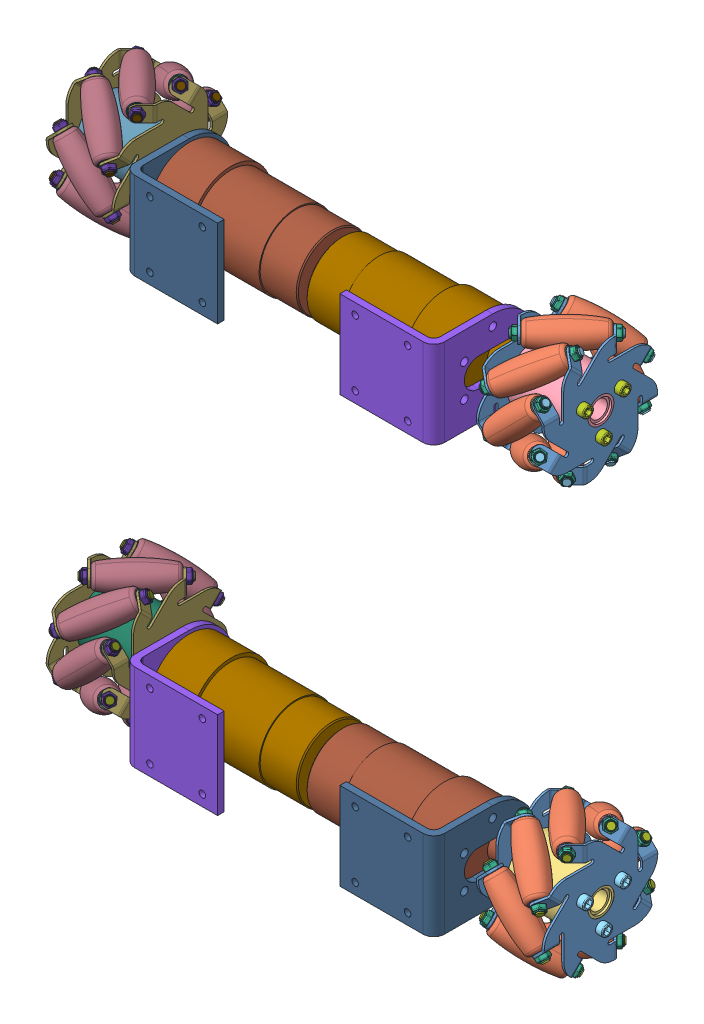
SolidWorks assembly car, configuration 默认. Lengths in mm. (continued)
Components (placement in the parent): (continued)
- Tank(2)^car-1: Tank(2)^car [默认] at origin size (280 382.88 170.83) (virtual) (continued)
  - Mecanum_Wheel_60mm_Left_ASM_AP214 v1 (1)^Tank(2)_car-1: Mecanum_Wheel_60mm_Left_ASM_AP214 v1 (1)^Tank(2)_car [默认] at (89.5247 -221.4281 -134.5883) x (1 0 0) z (0 -0.707107 -0.707107) size (37 63.14 63.14) (virtual) (continued)
    - roller_Varsayilan (1)^Mecanum_Wheel_60mm_Left_ASM_AP214 v1 (1)_Tank(2)_car-2: roller_Varsayilan (1)^Mecanum_Wheel_60mm_Left_ASM_AP214 v1 (1)_Tank(2)_car [默认] at (-11.1205 22.2762 30.2518) x (0.707107 0 0.707107) z (-0.228848 -0.94618 0.228848) size (29.8 12.94 12.94) (virtual)
    - roller_Varsayilan (1)^Mecanum_Wheel_60mm_Left_ASM_AP214 v1 (1)_Tank(2)_car-3: roller_Varsayilan (1)^Mecanum_Wheel_60mm_Left_ASM_AP214 v1 (1)_Tank(2)_car [默认] at (-11.1205 15.7922 13.8838) x (0.707107 0.5 0.5) z (-0.228848 -0.50723 0.830871) size (29.8 12.94 12.94) (virtual)
    - roller_Varsayilan (1)^Mecanum_Wheel_60mm_Left_ASM_AP214 v1 (1)_Tank(2)_car-4: roller_Varsayilan (1)^Mecanum_Wheel_60mm_Left_ASM_AP214 v1 (1)_Tank(2)_car [默认] at (-11.1205 -0.3667 6.8948) x (0.707107 0.707107 0) z (-0.228848 0.228848 0.94618) size (29.8 12.94 12.94) (virtual)
    - roller_Varsayilan (1)^Mecanum_Wheel_60mm_Left_ASM_AP214 v1 (1)_Tank(2)_car-5: roller_Varsayilan (1)^Mecanum_Wheel_60mm_Left_ASM_AP214 v1 (1)_Tank(2)_car [默认] at (-11.1205 -16.7348 13.3789) x (0.707107 0.5 -0.5) z (-0.228848 0.830871 0.50723) size (29.8 12.94 12.94) (virtual)
    - roller_Varsayilan (1)^Mecanum_Wheel_60mm_Left_ASM_AP214 v1 (1)_Tank(2)_car-6: roller_Varsayilan (1)^Mecanum_Wheel_60mm_Left_ASM_AP214 v1 (1)_Tank(2)_car [默认] at (-11.1205 -23.7238 29.5377) x (0.707107 0 -0.707107) z (-0.228848 0.94618 -0.228848) size (29.8 12.94 12.94) (virtual)
    - roller_Varsayilan (1)^Mecanum_Wheel_60mm_Left_ASM_AP214 v1 (1)_Tank(2)_car-7: roller_Varsayilan (1)^Mecanum_Wheel_60mm_Left_ASM_AP214 v1 (1)_Tank(2)_car [默认] at (-11.1205 -17.2397 45.9058) x (0.707107 -0.5 -0.5) z (-0.228848 0.50723 -0.830871) size (29.8 12.94 12.94) (virtual)
    - roller_Varsayilan (1)^Mecanum_Wheel_60mm_Left_ASM_AP214 v1 (1)_Tank(2)_car-8: roller_Varsayilan (1)^Mecanum_Wheel_60mm_Left_ASM_AP214 v1 (1)_Tank(2)_car [默认] at (-11.1205 -1.0808 52.8948) x (0.707107 -0.707107 0) z (-0.228848 -0.228848 -0.94618) size (29.8 12.94 12.94) (virtual)
    - 3x35_screw_Varsayilan (1)^Mecanum_Wheel_60mm_Left_ASM_AP214 v1 (1)_Tank(2)_car-2: 3x35_screw_Varsayilan (1)^Mecanum_Wheel_60mm_Left_ASM_AP214 v1 (1)_Tank(2)_car [默认] at (-29.9304 1.8644 20.2355) x (0 -0.866025 0.5) z (1 0 0) size (5 5 37) (virtual)
    - 3x35_screw_Varsayilan (1)^Mecanum_Wheel_60mm_Left_ASM_AP214 v1 (1)_Tank(2)_car-3: 3x35_screw_Varsayilan (1)^Mecanum_Wheel_60mm_Left_ASM_AP214 v1 (1)_Tank(2)_car [默认] at (-29.9304 -10.383 32.483) x (0 0.866025 0.5) z (1 0 0) size (5 5 37) (virtual)
    - 3mm_bolt_Varsayilan (1)^Mecanum_Wheel_60mm_Left_ASM_AP214 v1 (1)_Tank(2)_car-2: 3mm_bolt_Varsayilan (1)^Mecanum_Wheel_60mm_Left_ASM_AP214 v1 (1)_Tank(2)_car [默认] at (-27.0247 -10.383 32.483) x (0 -0.940173 -0.340697) z (-1 0 0) size (5.6 5.2 2.5) (virtual)
    - 3mm_bolt_Varsayilan (1)^Mecanum_Wheel_60mm_Left_ASM_AP214 v1 (1)_Tank(2)_car-3: 3mm_bolt_Varsayilan (1)^Mecanum_Wheel_60mm_Left_ASM_AP214 v1 (1)_Tank(2)_car [默认] at (-27.0247 6.3473 36.9659) x (0 0.175035 0.984562) z (-1 0 0) size (5.6 5.2 2.5) (virtual)
    - 3mm_bolt_Varsayilan (1)^Mecanum_Wheel_60mm_Left_ASM_AP214 v1 (1)_Tank(2)_car-4: 3mm_bolt_Varsayilan (1)^Mecanum_Wheel_60mm_Left_ASM_AP214 v1 (1)_Tank(2)_car [默认] at (-22.8133 7.5242 5.6158) x (-0.060636 0.747379 -0.661626) z (-0.707107 -0.5 -0.5) size (5.6 5.2 2.5) (virtual)
    - 3mm_bolt_Varsayilan (1)^Mecanum_Wheel_60mm_Left_ASM_AP214 v1 (1)_Tank(2)_car-5: 3mm_bolt_Varsayilan (1)^Mecanum_Wheel_60mm_Left_ASM_AP214 v1 (1)_Tank(2)_car [默认] at (-0.1419 23.5552 21.6469) x (0.267213 0.465725 -0.843622) z (0.707107 0.5 0.5) size (5.6 5.2 2.5) (virtual)
    - 3mm_bolt_Varsayilan (1)^Mecanum_Wheel_60mm_Left_ASM_AP214 v1 (1)_Tank(2)_car-6: 3mm_bolt_Varsayilan (1)^Mecanum_Wheel_60mm_Left_ASM_AP214 v1 (1)_Tank(2)_car [默认] at (-22.8133 22.2762 18.5591) x (-0.060636 0.996316 0.060636) z (-0.707107 0 -0.707107) size (5.6 5.2 2.5) (virtual)
    - 3mm_bolt_Varsayilan (1)^Mecanum_Wheel_60mm_Left_ASM_AP214 v1 (1)_Tank(2)_car-7: 3mm_bolt_Varsayilan (1)^Mecanum_Wheel_60mm_Left_ASM_AP214 v1 (1)_Tank(2)_car [默认] at (-22.8133 23.5552 38.1427) x (-0.060636 0.661626 0.747379) z (-0.707107 0.5 -0.5) size (5.6 5.2 2.5) (virtual)
    - 3mm_bolt_Varsayilan (1)^Mecanum_Wheel_60mm_Left_ASM_AP214 v1 (1)_Tank(2)_car-8: 3mm_bolt_Varsayilan (1)^Mecanum_Wheel_60mm_Left_ASM_AP214 v1 (1)_Tank(2)_car [默认] at (-22.8133 10.6119 52.8948) x (-0.060636 -0.060636 0.996316) z (-0.707107 0.707107 0) size (5.6 5.2 2.5) (virtual)
    - 3mm_bolt_Varsayilan (1)^Mecanum_Wheel_60mm_Left_ASM_AP214 v1 (1)_Tank(2)_car-9: 3mm_bolt_Varsayilan (1)^Mecanum_Wheel_60mm_Left_ASM_AP214 v1 (1)_Tank(2)_car [默认] at (-22.8133 -8.9717 54.1738) x (-0.060636 -0.747379 0.661626) z (-0.707107 0.5 0.5) size (5.6 5.2 2.5) (virtual)
    - 3mm_bolt_Varsayilan (1)^Mecanum_Wheel_60mm_Left_ASM_AP214 v1 (1)_Tank(2)_car-10: 3mm_bolt_Varsayilan (1)^Mecanum_Wheel_60mm_Left_ASM_AP214 v1 (1)_Tank(2)_car [默认] at (-22.8133 -23.7238 41.2305) x (-0.060636 -0.996316 -0.060636) z (-0.707107 0 0.707107) size (5.6 5.2 2.5) (virtual)
    - 3mm_bolt_Varsayilan (1)^Mecanum_Wheel_60mm_Left_ASM_AP214 v1 (1)_Tank(2)_car-11: 3mm_bolt_Varsayilan (1)^Mecanum_Wheel_60mm_Left_ASM_AP214 v1 (1)_Tank(2)_car [默认] at (-22.8133 -25.0028 21.6469) x (-0.060636 -0.661626 -0.747379) z (-0.707107 -0.5 0.5) size (5.6 5.2 2.5) (virtual)
    - 3mm_bolt_Varsayilan (1)^Mecanum_Wheel_60mm_Left_ASM_AP214 v1 (1)_Tank(2)_car-12: 3mm_bolt_Varsayilan (1)^Mecanum_Wheel_60mm_Left_ASM_AP214 v1 (1)_Tank(2)_car [默认] at (-22.8133 -12.0594 6.8948) x (-0.060636 0.060636 -0.996316) z (-0.707107 -0.707107 0) size (5.6 5.2 2.5) (virtual)
    - 3mm_bolt_Varsayilan (1)^Mecanum_Wheel_60mm_Left_ASM_AP214 v1 (1)_Tank(2)_car-13: 3mm_bolt_Varsayilan (1)^Mecanum_Wheel_60mm_Left_ASM_AP214 v1 (1)_Tank(2)_car [默认] at (-0.1419 22.2762 41.2305) x (0.267213 0.925848 -0.267213) z (0.707107 0 0.707107) size (5.6 5.2 2.5) (virtual)
    - 3mm_bolt_Varsayilan (1)^Mecanum_Wheel_60mm_Left_ASM_AP214 v1 (1)_Tank(2)_car-14: 3mm_bolt_Varsayilan (1)^Mecanum_Wheel_60mm_Left_ASM_AP214 v1 (1)_Tank(2)_car [默认] at (-0.1419 7.5242 54.1738) x (0.267213 0.843622 0.465725) z (0.707107 -0.5 0.5) size (5.6 5.2 2.5) (virtual)
    - 3mm_bolt_Varsayilan (1)^Mecanum_Wheel_60mm_Left_ASM_AP214 v1 (1)_Tank(2)_car-15: 3mm_bolt_Varsayilan (1)^Mecanum_Wheel_60mm_Left_ASM_AP214 v1 (1)_Tank(2)_car [默认] at (-0.1419 -12.0594 52.8948) x (0.267213 0.267213 0.925848) z (0.707107 -0.707107 0) size (5.6 5.2 2.5) (virtual)
    - 3mm_bolt_Varsayilan (1)^Mecanum_Wheel_60mm_Left_ASM_AP214 v1 (1)_Tank(2)_car-16: 3mm_bolt_Varsayilan (1)^Mecanum_Wheel_60mm_Left_ASM_AP214 v1 (1)_Tank(2)_car [默认] at (-0.1419 -25.0028 38.1427) x (0.267213 -0.465725 0.843622) z (0.707107 -0.5 -0.5) size (5.6 5.2 2.5) (virtual)
    - 3mm_bolt_Varsayilan (1)^Mecanum_Wheel_60mm_Left_ASM_AP214 v1 (1)_Tank(2)_car-17: 3mm_bolt_Varsayilan (1)^Mecanum_Wheel_60mm_Left_ASM_AP214 v1 (1)_Tank(2)_car [默认] at (-0.1419 -23.7238 18.5591) x (0.267213 -0.925848 0.267213) z (0.707107 0 -0.707107) size (5.6 5.2 2.5) (virtual)
    - 3mm_bolt_Varsayilan (1)^Mecanum_Wheel_60mm_Left_ASM_AP214 v1 (1)_Tank(2)_car-18: 3mm_bolt_Varsayilan (1)^Mecanum_Wheel_60mm_Left_ASM_AP214 v1 (1)_Tank(2)_car [默认] at (-0.1419 -8.9717 5.6158) x (0.267213 -0.843622 -0.465725) z (0.707107 0.5 -0.5) size (5.6 5.2 2.5) (virtual)
    - 3mm_bolt_Varsayilan (1)^Mecanum_Wheel_60mm_Left_ASM_AP214 v1 (1)_Tank(2)_car-19: 3mm_bolt_Varsayilan (1)^Mecanum_Wheel_60mm_Left_ASM_AP214 v1 (1)_Tank(2)_car [默认] at (-0.1419 10.6119 6.8948) x (0.267213 -0.267213 -0.925848) z (0.707107 0.707107 0) size (5.6 5.2 2.5) (virtual)
    - two_sided_screw_Varsayilan (1)^Mecanum_Wheel_60mm_Left_ASM_AP214 v1 (1)_Tank(2)_car-2: two_sided_screw_Varsayilan (1)^Mecanum_Wheel_60mm_Left_ASM_AP214 v1 (1)_Tank(2)_car [默认] at (-24.8906 22.2762 16.4817) x (-0.576606 0.578837 0.576606) z (0.707107 0 0.707107) size (3 3 38) (virtual)
    - two_sided_screw_Varsayilan (1)^Mecanum_Wheel_60mm_Left_ASM_AP214 v1 (1)_Tank(2)_car-3: two_sided_screw_Varsayilan (1)^Mecanum_Wheel_60mm_Left_ASM_AP214 v1 (1)_Tank(2)_car [默认] at (-24.8906 25.0242 36.6738) x (-0.576606 0.001578 0.817021) z (0.707107 -0.5 0.5) size (3 3 38) (virtual)
    - two_sided_screw_Varsayilan (1)^Mecanum_Wheel_60mm_Left_ASM_AP214 v1 (1)_Tank(2)_car-4: two_sided_screw_Varsayilan (1)^Mecanum_Wheel_60mm_Left_ASM_AP214 v1 (1)_Tank(2)_car [默认] at (-24.8906 12.6893 52.8948) x (-0.576606 -0.576606 0.578837) z (0.707107 -0.707107 0) size (3 3 38) (virtual)
    - two_sided_screw_Varsayilan (1)^Mecanum_Wheel_60mm_Left_ASM_AP214 v1 (1)_Tank(2)_car-5: two_sided_screw_Varsayilan (1)^Mecanum_Wheel_60mm_Left_ASM_AP214 v1 (1)_Tank(2)_car [默认] at (-24.8906 -7.5028 55.6427) x (-0.576606 -0.817021 0.001578) z (0.707107 -0.5 -0.5) size (3 3 38) (virtual)
    - two_sided_screw_Varsayilan (1)^Mecanum_Wheel_60mm_Left_ASM_AP214 v1 (1)_Tank(2)_car-6: two_sided_screw_Varsayilan (1)^Mecanum_Wheel_60mm_Left_ASM_AP214 v1 (1)_Tank(2)_car [默认] at (-24.8906 -23.7238 43.3078) x (-0.576606 -0.578837 -0.576606) z (0.707107 0 -0.707107) size (3 3 38) (virtual)
    - two_sided_screw_Varsayilan (1)^Mecanum_Wheel_60mm_Left_ASM_AP214 v1 (1)_Tank(2)_car-7: two_sided_screw_Varsayilan (1)^Mecanum_Wheel_60mm_Left_ASM_AP214 v1 (1)_Tank(2)_car [默认] at (-24.8906 -26.4717 23.1158) x (-0.576606 -0.001578 -0.817021) z (0.707107 0.5 -0.5) size (3 3 38) (virtual)
    - two_sided_screw_Varsayilan (1)^Mecanum_Wheel_60mm_Left_ASM_AP214 v1 (1)_Tank(2)_car-8: two_sided_screw_Varsayilan (1)^Mecanum_Wheel_60mm_Left_ASM_AP214 v1 (1)_Tank(2)_car [默认] at (-24.8906 -14.1368 6.8948) x (-0.576606 0.576606 -0.578837) z (0.707107 0.707107 0) size (3 3 38) (virtual)
  - DC LF (1)^Tank(2)_car-1: DC LF (1)^Tank(2)_car [默认] at (-41 -242.0551 -178.2389) x (-1 0 0) z (0 0 1) size (95 40 47) (virtual)
    - Component10(Mirror)^DC LF (1)_Tank(2)_car-1: Component10(Mirror)^DC LF (1)_Tank(2)_car [默认] at origin size (43 40 47) (virtual)
    - DC LF (1)-2^DC LF (1)_Tank(2)_car-1: DC LF (1)-2^DC LF (1)_Tank(2)_car [默认] at origin size (95 37 37) (virtual)
  - DC RF (1)^Tank(2)_car-1: DC RF (1)^Tank(2)_car [默认] at (0 -242.0551 -178.2389) x (1 0 0) z (0 0 -1) size (95 40 47) (virtual)
    - Component10^DC RF (1)_Tank(2)_car-1: Component10^DC RF (1)_Tank(2)_car [默认] at origin size (43 40 47) (virtual)
    - DC RF (1)-3^DC RF (1)_Tank(2)_car-1: DC RF (1)-3^DC RF (1)_Tank(2)_car [默认] at origin size (95 37 37) (virtual)
  - Mecanum_Wheel_60mm_Right_ASM_AP214 v1 (1)^Tank(2)_car-1: Mecanum_Wheel_60mm_Right_ASM_AP214 v1 (1)^Tank(2)_car [默认] at (-134.5 -218.5276 -89.1195) x (1 0 0) z (0 0 -1) size (83 63.25 63.25) (virtual)
    - plate_2_Varsayilan^Mecanum_Wheel_60mm_Right_ASM_AP214 v1 (1)_Tank(2)_car-1: plate_2_Varsayilan^Mecanum_Wheel_60mm_Right_ASM_AP214 v1 (1)_Tank(2)_car [默认] at (56.8037 4.8798 97.2247) x (0.707107 0.707107 0) z (0 0 1) size (41.63 41.63 53.77) (virtual)
    - roller_Varsayilan^Mecanum_Wheel_60mm_Right_ASM_AP214 v1 (1)_Tank(2)_car-1: roller_Varsayilan^Mecanum_Wheel_60mm_Right_ASM_AP214 v1 (1)_Tank(2)_car [默认] at (15.1622 40.0059 51.0708) x (-0.707107 0.5 0.5) z (-0.704237 -0.434326 -0.561615) size (29.8 12.94 12.94) (virtual)
    - liner_Varsayilan^Mecanum_Wheel_60mm_Right_ASM_AP214 v1 (1)_Tank(2)_car-1: liner_Varsayilan^Mecanum_Wheel_60mm_Right_ASM_AP214 v1 (1)_Tank(2)_car [默认] at (4.8906 47.2689 58.3339) x (-0.663539 -0.224823 -0.713562) z (-0.24437 -0.836334 0.490743) size (7 1 7) (virtual)
    - inner_cylinder_Varsayilan^Mecanum_Wheel_60mm_Right_ASM_AP214 v1 (1)_Tank(2)_car-1: inner_cylinder_Varsayilan^Mecanum_Wheel_60mm_Right_ASM_AP214 v1 (1)_Tank(2)_car [默认] at (30 23.5276 67.1195) x (0 0 1) z (-1 0 0) size (26 26 31) (virtual)
    - two_sided_screw_Varsayilan^Mecanum_Wheel_60mm_Right_ASM_AP214 v1 (1)_Tank(2)_car-1: two_sided_screw_Varsayilan^Mecanum_Wheel_60mm_Right_ASM_AP214 v1 (1)_Tank(2)_car [默认] at (28.9323 30.2689 41.3339) x (-0.195015 0.541787 -0.817579) z (-0.707107 0.5 0.5) size (3 3 38) (virtual)
    - 3mm_bolt_Varsayilan^Mecanum_Wheel_60mm_Right_ASM_AP214 v1 (1)_Tank(2)_car-1: 3mm_bolt_Varsayilan^Mecanum_Wheel_60mm_Right_ASM_AP214 v1 (1)_Tank(2)_car [默认] at (4.155 47.7891 58.854) x (0.638071 0.755922 0.146447) z (-0.707107 0.5 0.5) size (5.6 5.2 2.5) (virtual)
    - 3x35_screw_Varsayilan^Mecanum_Wheel_60mm_Right_ASM_AP214 v1 (1)_Tank(2)_car-1: 3x35_screw_Varsayilan^Mecanum_Wheel_60mm_Right_ASM_AP214 v1 (1)_Tank(2)_car [默认] at (-3 18.5276 58.4592) x (0 0.745603 -0.666391) z (1 0 0) size (5 5 37) (virtual)
    - plate_2_Varsayilan^Mecanum_Wheel_60mm_Right_ASM_AP214 v1 (1)_Tank(2)_car-2: plate_2_Varsayilan^Mecanum_Wheel_60mm_Right_ASM_AP214 v1 (1)_Tank(2)_car [默认] at (-25.8037 4.8798 37.0142) x (-0.707107 0.707107 0) z (0 0 -1) size (41.63 41.63 53.77) (virtual)
    - liner_Varsayilan^Mecanum_Wheel_60mm_Right_ASM_AP214 v1 (1)_Tank(2)_car-2: liner_Varsayilan^Mecanum_Wheel_60mm_Right_ASM_AP214 v1 (1)_Tank(2)_car [默认] at (26.1038 32.2689 43.3339) x (0.54662 -0.062042 0.835079) z (-0.448561 -0.8638 0.22944) size (7 1 7) (virtual)
    - 3mm_bolt_Varsayilan^Mecanum_Wheel_60mm_Right_ASM_AP214 v1 (1)_Tank(2)_car-2: 3mm_bolt_Varsayilan^Mecanum_Wheel_60mm_Right_ASM_AP214 v1 (1)_Tank(2)_car [默认] at (26.8109 31.7689 42.8339) x (0.358192 -0.356391 0.862951) z (0.707107 -0.5 -0.5) size (5.6 5.2 2.5) (virtual)
    - 3mm_bolt_Varsayilan^Mecanum_Wheel_60mm_Right_ASM_AP214 v1 (1)_Tank(2)_car-3: 3mm_bolt_Varsayilan^Mecanum_Wheel_60mm_Right_ASM_AP214 v1 (1)_Tank(2)_car [默认] at (0 18.5276 75.7797) x (0 -0.80734 0.590087) z (-1 0 0) size (5.6 5.2 2.5) (virtual)
    - 3x35_screw_Varsayilan^Mecanum_Wheel_60mm_Right_ASM_AP214 v1 (1)_Tank(2)_car-2: 3x35_screw_Varsayilan^Mecanum_Wheel_60mm_Right_ASM_AP214 v1 (1)_Tank(2)_car [默认] at (-3 18.5276 75.7797) x (0 -0.949913 -0.312516) z (1 0 0) size (5 5 37) (virtual)
    - 3x35_screw_Varsayilan^Mecanum_Wheel_60mm_Right_ASM_AP214 v1 (1)_Tank(2)_car-3: 3x35_screw_Varsayilan^Mecanum_Wheel_60mm_Right_ASM_AP214 v1 (1)_Tank(2)_car [默认] at (-3 33.5276 67.1195) x (0 0.20431 0.978906) z (1 0 0) size (5 5 37) (virtual)
    - 3mm_bolt_Varsayilan^Mecanum_Wheel_60mm_Right_ASM_AP214 v1 (1)_Tank(2)_car-4: 3mm_bolt_Varsayilan^Mecanum_Wheel_60mm_Right_ASM_AP214 v1 (1)_Tank(2)_car [默认] at (0 33.5276 67.1195) x (0 0.9147 0.404133) z (-1 0 0) size (5.6 5.2 2.5) (virtual)
    - 3mm_bolt_Varsayilan^Mecanum_Wheel_60mm_Right_ASM_AP214 v1 (1)_Tank(2)_car-5: 3mm_bolt_Varsayilan^Mecanum_Wheel_60mm_Right_ASM_AP214 v1 (1)_Tank(2)_car [默认] at (0 18.5276 58.4592) x (0 -0.107361 -0.99422) z (-1 0 0) size (5.6 5.2 2.5) (virtual)
    - two_sided_screw_Varsayilan^Mecanum_Wheel_60mm_Right_ASM_AP214 v1 (1)_Tank(2)_car-2: two_sided_screw_Varsayilan^Mecanum_Wheel_60mm_Right_ASM_AP214 v1 (1)_Tank(2)_car [默认] at (28.9323 10.0613 44.1195) x (-0.195015 -0.195015 -0.961217) z (-0.707107 0.707107 0) size (3 3 38) (virtual)
    - two_sided_screw_Varsayilan^Mecanum_Wheel_60mm_Right_ASM_AP214 v1 (1)_Tank(2)_car-3: two_sided_screw_Varsayilan^Mecanum_Wheel_60mm_Right_ASM_AP214 v1 (1)_Tank(2)_car [默认] at (28.9323 -2.258 60.3781) x (-0.195015 -0.817579 -0.541787) z (-0.707107 0.5 -0.5) size (3 3 38) (virtual)
    - two_sided_screw_Varsayilan^Mecanum_Wheel_60mm_Right_ASM_AP214 v1 (1)_Tank(2)_car-4: two_sided_screw_Varsayilan^Mecanum_Wheel_60mm_Right_ASM_AP214 v1 (1)_Tank(2)_car [默认] at (28.9323 0.5276 80.5857) x (-0.195015 -0.961217 0.195015) z (-0.707107 0 -0.707107) size (3 3 38) (virtual)
    - two_sided_screw_Varsayilan^Mecanum_Wheel_60mm_Right_ASM_AP214 v1 (1)_Tank(2)_car-5: two_sided_screw_Varsayilan^Mecanum_Wheel_60mm_Right_ASM_AP214 v1 (1)_Tank(2)_car [默认] at (28.9323 16.7862 92.905) x (-0.195015 -0.541787 0.817579) z (-0.707107 -0.5 -0.5) size (3 3 38) (virtual)
    - two_sided_screw_Varsayilan^Mecanum_Wheel_60mm_Right_ASM_AP214 v1 (1)_Tank(2)_car-6: two_sided_screw_Varsayilan^Mecanum_Wheel_60mm_Right_ASM_AP214 v1 (1)_Tank(2)_car [默认] at (28.9323 36.9938 90.1195) x (-0.195015 0.195015 0.961217) z (-0.707107 -0.707107 0) size (3 3 38) (virtual)
    - two_sided_screw_Varsayilan^Mecanum_Wheel_60mm_Right_ASM_AP214 v1 (1)_Tank(2)_car-7: two_sided_screw_Varsayilan^Mecanum_Wheel_60mm_Right_ASM_AP214 v1 (1)_Tank(2)_car [默认] at (28.9323 49.3131 73.8608) x (-0.195015 0.817579 0.541787) z (-0.707107 -0.5 0.5) size (3 3 38) (virtual)
    - two_sided_screw_Varsayilan^Mecanum_Wheel_60mm_Right_ASM_AP214 v1 (1)_Tank(2)_car-8: two_sided_screw_Varsayilan^Mecanum_Wheel_60mm_Right_ASM_AP214 v1 (1)_Tank(2)_car [默认] at (28.9323 46.5276 53.6532) x (-0.195015 0.961217 -0.195015) z (-0.707107 0 0.707107) size (3 3 38) (virtual)
    - 3mm_bolt_Varsayilan^Mecanum_Wheel_60mm_Right_ASM_AP214 v1 (1)_Tank(2)_car-6: 3mm_bolt_Varsayilan^Mecanum_Wheel_60mm_Right_ASM_AP214 v1 (1)_Tank(2)_car [默认] at (26.8109 12.1826 44.1195) x (0.358192 0.358192 0.862205) z (0.707107 -0.707107 0) size (5.6 5.2 2.5) (virtual)
    - 3mm_bolt_Varsayilan^Mecanum_Wheel_60mm_Right_ASM_AP214 v1 (1)_Tank(2)_car-7: 3mm_bolt_Varsayilan^Mecanum_Wheel_60mm_Right_ASM_AP214 v1 (1)_Tank(2)_car [默认] at (26.8109 -0.758 58.8781) x (0.358192 0.862951 0.356391) z (0.707107 -0.5 0.5) size (5.6 5.2 2.5) (virtual)
    - 3mm_bolt_Varsayilan^Mecanum_Wheel_60mm_Right_ASM_AP214 v1 (1)_Tank(2)_car-8: 3mm_bolt_Varsayilan^Mecanum_Wheel_60mm_Right_ASM_AP214 v1 (1)_Tank(2)_car [默认] at (26.8109 0.5276 78.4644) x (0.358192 0.862205 -0.358192) z (0.707107 0 0.707107) size (5.6 5.2 2.5) (virtual)
    - 3mm_bolt_Varsayilan^Mecanum_Wheel_60mm_Right_ASM_AP214 v1 (1)_Tank(2)_car-9: 3mm_bolt_Varsayilan^Mecanum_Wheel_60mm_Right_ASM_AP214 v1 (1)_Tank(2)_car [默认] at (26.8109 15.2862 91.405) x (0.358192 0.356391 -0.862951) z (0.707107 0.5 0.5) size (5.6 5.2 2.5) (virtual)
    - 3mm_bolt_Varsayilan^Mecanum_Wheel_60mm_Right_ASM_AP214 v1 (1)_Tank(2)_car-10: 3mm_bolt_Varsayilan^Mecanum_Wheel_60mm_Right_ASM_AP214 v1 (1)_Tank(2)_car [默认] at (26.8109 34.8725 90.1195) x (0.358192 -0.358192 -0.862205) z (0.707107 0.707107 0) size (5.6 5.2 2.5) (virtual)
    - 3mm_bolt_Varsayilan^Mecanum_Wheel_60mm_Right_ASM_AP214 v1 (1)_Tank(2)_car-11: 3mm_bolt_Varsayilan^Mecanum_Wheel_60mm_Right_ASM_AP214 v1 (1)_Tank(2)_car [默认] at (26.8109 47.8131 75.3608) x (0.358192 -0.862951 -0.356391) z (0.707107 0.5 -0.5) size (5.6 5.2 2.5) (virtual)
    - 3mm_bolt_Varsayilan^Mecanum_Wheel_60mm_Right_ASM_AP214 v1 (1)_Tank(2)_car-12: 3mm_bolt_Varsayilan^Mecanum_Wheel_60mm_Right_ASM_AP214 v1 (1)_Tank(2)_car [默认] at (26.8109 46.5276 55.7745) x (0.358192 -0.862205 0.358192) z (0.707107 0 -0.707107) size (5.6 5.2 2.5) (virtual)
    - 3mm_bolt_Varsayilan^Mecanum_Wheel_60mm_Right_ASM_AP214 v1 (1)_Tank(2)_car-13: 3mm_bolt_Varsayilan^Mecanum_Wheel_60mm_Right_ASM_AP214 v1 (1)_Tank(2)_car [默认] at (4.155 34.8385 44.1195) x (0.638071 0.638071 -0.430964) z (-0.707107 0.707107 0) size (5.6 5.2 2.5) (virtual)
    - 3mm_bolt_Varsayilan^Mecanum_Wheel_60mm_Right_ASM_AP214 v1 (1)_Tank(2)_car-14: 3mm_bolt_Varsayilan^Mecanum_Wheel_60mm_Right_ASM_AP214 v1 (1)_Tank(2)_car [默认] at (4.155 15.2622 42.858) x (0.638071 0.146447 -0.755922) z (-0.707107 0.5 -0.5) size (5.6 5.2 2.5) (virtual)
    - 3mm_bolt_Varsayilan^Mecanum_Wheel_60mm_Right_ASM_AP214 v1 (1)_Tank(2)_car-15: 3mm_bolt_Varsayilan^Mecanum_Wheel_60mm_Right_ASM_AP214 v1 (1)_Tank(2)_car [默认] at (4.155 0.5276 55.8085) x (0.638071 -0.430964 -0.638071) z (-0.707107 0 -0.707107) size (5.6 5.2 2.5) (virtual)
    - 3mm_bolt_Varsayilan^Mecanum_Wheel_60mm_Right_ASM_AP214 v1 (1)_Tank(2)_car-16: 3mm_bolt_Varsayilan^Mecanum_Wheel_60mm_Right_ASM_AP214 v1 (1)_Tank(2)_car [默认] at (4.155 -0.7339 75.3849) x (0.638071 -0.755922 -0.146447) z (-0.707107 -0.5 -0.5) size (5.6 5.2 2.5) (virtual)
    - 3mm_bolt_Varsayilan^Mecanum_Wheel_60mm_Right_ASM_AP214 v1 (1)_Tank(2)_car-17: 3mm_bolt_Varsayilan^Mecanum_Wheel_60mm_Right_ASM_AP214 v1 (1)_Tank(2)_car [默认] at (4.155 12.2166 90.1195) x (0.638071 -0.638071 0.430964) z (-0.707107 -0.707107 0) size (5.6 5.2 2.5) (virtual)
    - 3mm_bolt_Varsayilan^Mecanum_Wheel_60mm_Right_ASM_AP214 v1 (1)_Tank(2)_car-18: 3mm_bolt_Varsayilan^Mecanum_Wheel_60mm_Right_ASM_AP214 v1 (1)_Tank(2)_car [默认] at (4.155 31.793 91.381) x (0.638071 -0.146447 0.755922) z (-0.707107 -0.5 0.5) size (5.6 5.2 2.5) (virtual)
    - 3mm_bolt_Varsayilan^Mecanum_Wheel_60mm_Right_ASM_AP214 v1 (1)_Tank(2)_car-19: 3mm_bolt_Varsayilan^Mecanum_Wheel_60mm_Right_ASM_AP214 v1 (1)_Tank(2)_car [默认] at (4.155 46.5276 78.4304) x (0.638071 0.430964 0.638071) z (-0.707107 0 0.707107) size (5.6 5.2 2.5) (virtual)
    - liner_Varsayilan^Mecanum_Wheel_60mm_Right_ASM_AP214 v1 (1)_Tank(2)_car-3: liner_Varsayilan^Mecanum_Wheel_60mm_Right_ASM_AP214 v1 (1)_Tank(2)_car [默认] at (26.1038 12.8897 44.1195) x (0.54662 0.54662 0.634361) z (-0.448561 -0.448561 0.773037) size (7 1 7) (virtual)
    - liner_Varsayilan^Mecanum_Wheel_60mm_Right_ASM_AP214 v1 (1)_Tank(2)_car-4: liner_Varsayilan^Mecanum_Wheel_60mm_Right_ASM_AP214 v1 (1)_Tank(2)_car [默认] at (26.1038 -0.258 58.3781) x (0.54662 0.835079 0.062042) z (-0.448561 0.22944 0.8638) size (7 1 7) (virtual)
    - liner_Varsayilan^Mecanum_Wheel_60mm_Right_ASM_AP214 v1 (1)_Tank(2)_car-5: liner_Varsayilan^Mecanum_Wheel_60mm_Right_ASM_AP214 v1 (1)_Tank(2)_car [默认] at (26.1038 0.5276 77.7573) x (0.54662 0.634361 -0.54662) z (-0.448561 0.773037 0.448561) size (7 1 7) (virtual)
    - liner_Varsayilan^Mecanum_Wheel_60mm_Right_ASM_AP214 v1 (1)_Tank(2)_car-6: liner_Varsayilan^Mecanum_Wheel_60mm_Right_ASM_AP214 v1 (1)_Tank(2)_car [默认] at (26.1038 14.7862 90.905) x (0.54662 0.062042 -0.835079) z (-0.448561 0.8638 -0.22944) size (7 1 7) (virtual)
    - liner_Varsayilan^Mecanum_Wheel_60mm_Right_ASM_AP214 v1 (1)_Tank(2)_car-7: liner_Varsayilan^Mecanum_Wheel_60mm_Right_ASM_AP214 v1 (1)_Tank(2)_car [默认] at (26.1038 34.1654 90.1195) x (0.54662 -0.54662 -0.634361) z (-0.448561 0.448561 -0.773037) size (7 1 7) (virtual)
    - liner_Varsayilan^Mecanum_Wheel_60mm_Right_ASM_AP214 v1 (1)_Tank(2)_car-8: liner_Varsayilan^Mecanum_Wheel_60mm_Right_ASM_AP214 v1 (1)_Tank(2)_car [默认] at (26.1038 47.3131 75.8608) x (0.54662 -0.835079 -0.062042) z (-0.448561 -0.22944 -0.8638) size (7 1 7) (virtual)
    - liner_Varsayilan^Mecanum_Wheel_60mm_Right_ASM_AP214 v1 (1)_Tank(2)_car-9: liner_Varsayilan^Mecanum_Wheel_60mm_Right_ASM_AP214 v1 (1)_Tank(2)_car [默认] at (26.1038 46.5276 56.4816) x (0.54662 -0.634361 0.54662) z (-0.448561 -0.773037 -0.448561) size (7 1 7) (virtual)
    - liner_Varsayilan^Mecanum_Wheel_60mm_Right_ASM_AP214 v1 (1)_Tank(2)_car-10: liner_Varsayilan^Mecanum_Wheel_60mm_Right_ASM_AP214 v1 (1)_Tank(2)_car [默认] at (4.8906 34.1029 44.1195) x (-0.663539 -0.663539 -0.345591) z (-0.24437 -0.24437 0.938385) size (7 1 7) (virtual)
    - liner_Varsayilan^Mecanum_Wheel_60mm_Right_ASM_AP214 v1 (1)_Tank(2)_car-11: liner_Varsayilan^Mecanum_Wheel_60mm_Right_ASM_AP214 v1 (1)_Tank(2)_car [默认] at (4.8906 14.742 43.3781) x (-0.663539 -0.713562 0.224823) z (-0.24437 0.490743 0.836334) size (7 1 7) (virtual)
    - liner_Varsayilan^Mecanum_Wheel_60mm_Right_ASM_AP214 v1 (1)_Tank(2)_car-12: liner_Varsayilan^Mecanum_Wheel_60mm_Right_ASM_AP214 v1 (1)_Tank(2)_car [默认] at (4.8906 0.5276 56.5441) x (-0.663539 -0.345591 0.663539) z (-0.24437 0.938385 0.24437) size (7 1 7) (virtual)
    - liner_Varsayilan^Mecanum_Wheel_60mm_Right_ASM_AP214 v1 (1)_Tank(2)_car-13: liner_Varsayilan^Mecanum_Wheel_60mm_Right_ASM_AP214 v1 (1)_Tank(2)_car [默认] at (4.8906 -0.2138 75.905) x (-0.663539 0.224823 0.713562) z (-0.24437 0.836334 -0.490743) size (7 1 7) (virtual)
    - liner_Varsayilan^Mecanum_Wheel_60mm_Right_ASM_AP214 v1 (1)_Tank(2)_car-14: liner_Varsayilan^Mecanum_Wheel_60mm_Right_ASM_AP214 v1 (1)_Tank(2)_car [默认] at (4.8906 12.9522 90.1195) x (-0.663539 0.663539 0.345591) z (-0.24437 0.24437 -0.938385) size (7 1 7) (virtual)
    - liner_Varsayilan^Mecanum_Wheel_60mm_Right_ASM_AP214 v1 (1)_Tank(2)_car-15: liner_Varsayilan^Mecanum_Wheel_60mm_Right_ASM_AP214 v1 (1)_Tank(2)_car [默认] at (4.8906 32.3131 90.8608) x (-0.663539 0.713562 -0.224823) z (-0.24437 -0.490743 -0.836334) size (7 1 7) (virtual)
    - liner_Varsayilan^Mecanum_Wheel_60mm_Right_ASM_AP214 v1 (1)_Tank(2)_car-16: liner_Varsayilan^Mecanum_Wheel_60mm_Right_ASM_AP214 v1 (1)_Tank(2)_car [默认] at (4.8906 46.5276 77.6948) x (-0.663539 0.345591 -0.663539) z (-0.24437 -0.938385 -0.24437) size (7 1 7) (virtual)
    - roller_Varsayilan^Mecanum_Wheel_60mm_Right_ASM_AP214 v1 (1)_Tank(2)_car-2: roller_Varsayilan^Mecanum_Wheel_60mm_Right_ASM_AP214 v1 (1)_Tank(2)_car [默认] at (15.1622 23.8314 44.1195) x (-0.707107 0.707107 0) z (-0.704237 -0.704237 -0.090007) size (29.8 12.94 12.94) (virtual)
    - roller_Varsayilan^Mecanum_Wheel_60mm_Right_ASM_AP214 v1 (1)_Tank(2)_car-3: roller_Varsayilan^Mecanum_Wheel_60mm_Right_ASM_AP214 v1 (1)_Tank(2)_car [默认] at (15.1622 7.4789 50.6412) x (-0.707107 0.5 -0.5) z (-0.704237 -0.561615 0.434326) size (29.8 12.94 12.94) (virtual)
    - roller_Varsayilan^Mecanum_Wheel_60mm_Right_ASM_AP214 v1 (1)_Tank(2)_car-4: roller_Varsayilan^Mecanum_Wheel_60mm_Right_ASM_AP214 v1 (1)_Tank(2)_car [默认] at (15.1622 0.5276 66.8156) x (-0.707107 0 -0.707107) z (-0.704237 -0.090007 0.704237) size (29.8 12.94 12.94) (virtual)
    - roller_Varsayilan^Mecanum_Wheel_60mm_Right_ASM_AP214 v1 (1)_Tank(2)_car-5: roller_Varsayilan^Mecanum_Wheel_60mm_Right_ASM_AP214 v1 (1)_Tank(2)_car [默认] at (15.1622 7.0493 83.1681) x (-0.707107 -0.5 -0.5) z (-0.704237 0.434326 0.561615) size (29.8 12.94 12.94) (virtual)
    - roller_Varsayilan^Mecanum_Wheel_60mm_Right_ASM_AP214 v1 (1)_Tank(2)_car-6: roller_Varsayilan^Mecanum_Wheel_60mm_Right_ASM_AP214 v1 (1)_Tank(2)_car [默认] at (15.1622 23.2237 90.1195) x (-0.707107 -0.707107 0) z (-0.704237 0.704237 0.090007) size (29.8 12.94 12.94) (virtual)
    - roller_Varsayilan^Mecanum_Wheel_60mm_Right_ASM_AP214 v1 (1)_Tank(2)_car-7: roller_Varsayilan^Mecanum_Wheel_60mm_Right_ASM_AP214 v1 (1)_Tank(2)_car [默认] at (15.1622 39.5762 83.5977) x (-0.707107 -0.5 0.5) z (-0.704237 0.561615 -0.434326) size (29.8 12.94 12.94) (virtual)
    - roller_Varsayilan^Mecanum_Wheel_60mm_Right_ASM_AP214 v1 (1)_Tank(2)_car-8: roller_Varsayilan^Mecanum_Wheel_60mm_Right_ASM_AP214 v1 (1)_Tank(2)_car [默认] at (15.1622 46.5276 67.4233) x (-0.707107 0 0.707107) z (-0.704237 0.090007 -0.704237) size (29.8 12.94 12.94) (virtual)
  - Servo - Tower Pro MG995 v1^Tank(2)_car-1: Servo - Tower Pro MG995 v1^Tank(2)_car [默认] at (-20.1909 -105.9892 -168.1889) x (0 1 0) z (1 0 0) size (54.65 45.95 20) (hidden, virtual)
  - Servo - Tower Pro MG995 v1 (1)^Tank(2)_car-1: Servo - Tower Pro MG995 v1 (1)^Tank(2)_car [默认] at (-68.738 -167.5382 -77.5771) x (0 -1 0) z (0 0 1) size (54.65 45.95 20) (hidden, virtual)
  - Component28^Tank(2)_car-1: Component28^Tank(2)_car [默认] at origin size (156.84 188.14 67.67) (hidden, virtual)
  - Component29^Tank(2)_car-1: Component29^Tank(2)_car [默认] at origin size (155.3 279.55 56.21) (hidden, virtual)
  - Component30^Tank(2)_car-1: Component30^Tank(2)_car [默认] at (0 0.0008 -0.0012) x (1 0 0) z (0 0.000014 1) size (15 335.5 42.04) (hidden, virtual)
  - Component32^Tank(2)_car-1: Component32^Tank(2)_car [默认] at (-20.9352 -157.9705 -77.9961) x (-1 0 0) z (0 -0.870974 0.491329) size (5 22.25 12) (hidden, virtual)
  - Component34^Tank(2)_car-1: Component34^Tank(2)_car [默认] at (-8.75 -7.0417 -48.806) x (1 0 0) z (0 0.169017 0.985613) size (2.5 41.83 45.18) (hidden, virtual)
  - Component35^Tank(2)_car-1: Component35^Tank(2)_car [默认] at origin size (60 60 2) (hidden, virtual)
  - Component10_1^Tank(2)_car-1: Component10_1^Tank(2)_car [默认] at (430.9591 20.9358 250.8961) x (1 0 0) z (0 -1 0) size (20 4.8 20) (hidden, virtual)
  - Component36^Tank(2)_car-1: Component36^Tank(2)_car [默认] at origin size (3.02 8.83 2.5) (hidden, virtual)
  - Component37^Tank(2)_car-1: Component37^Tank(2)_car [默认] at origin size (3.05 8.83 2.5) (hidden, virtual)
  - Component38^Tank(2)_car-1: Component38^Tank(2)_car [默认] at origin size (3.05 8.83 2.5) (hidden, virtual)
